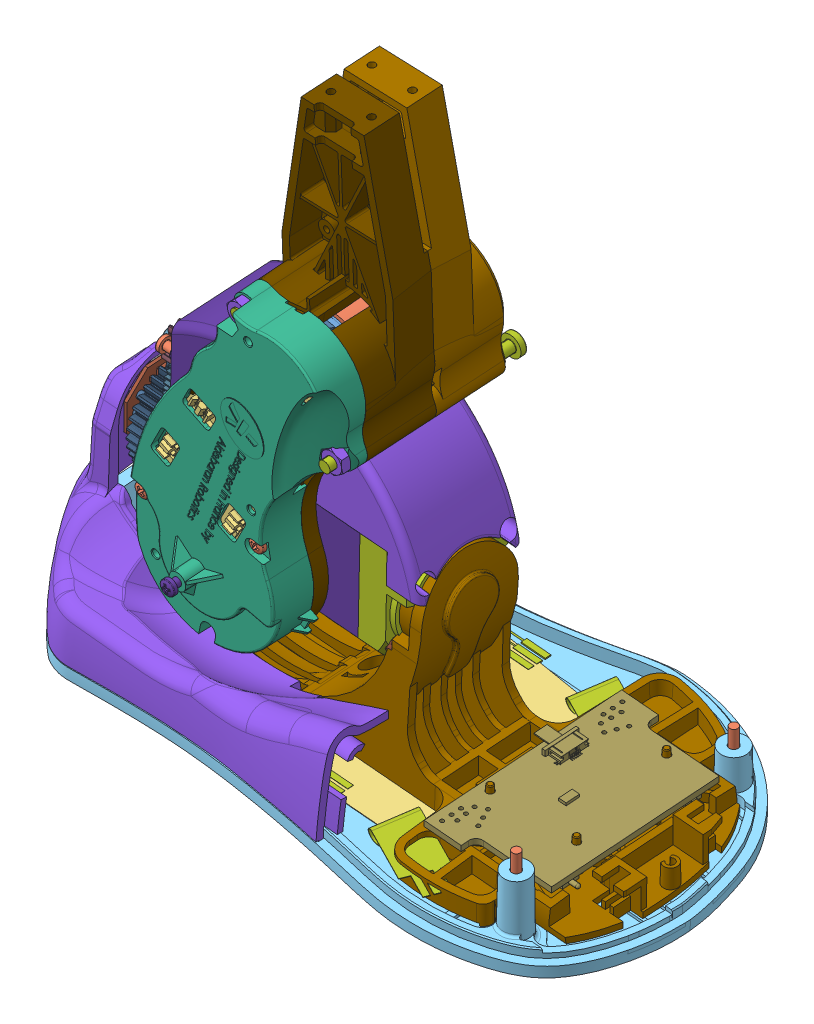
SolidWorks assembly Cheville_Gauche, configuration Défaut. Lengths in mm.
Overall size (176.95 178.66 110.8).
107 component instances, 54 part files, 21 mates.
Components (placement in the parent):
- Pied_Gauche-1: Pied_Gauche [Défaut] at (-33.6626 96.6362 176.8878) size (176.95 81.97 110.8)
  - Left_Foot_jambe droite-1: Left_Foot_jambe droite [Défaut] at (4.3479 -90.4053 5.2353) x (-0.007082 -0.079671 0.996796) z (-0.996073 0.088539 0) size (106.44 58.7 171.69)
    - STD_M850001__P_Scotch_double_Face_3M_5419_Default-1: STD_M850001__P_Scotch_double_Face_3M_5419_Default [Default] at (-23.9002 -40.8442 -61.9998) x (0 0 -1) z (0 1 0) size (13 10 0.25)
    - STD_M700004__PZ99_KA22x8_KA22 x 8-1: STD_M700004__PZ99_KA22x8_KA22 x 8 [Default] at (-16.4 -30.0842 45.1) x (0 1 0) z (-0.943584 0 -0.331134) size (9.5 3.9 3.91)
    - STD_M850001__P_Scotch_double_Face_3M_5419_Default-2: STD_M850001__P_Scotch_double_Face_3M_5419_Default [Default] at (27.1002 -40.5942 -74.9998) x (0 0 1) z (0 -1 0) size (13 10 0.25)
    - STD_E990013__P_FSR_4P-1: STD_E990013__P_FSR_4P [Default] at (19.0956 -40.8442 30.9044) x (0 0 1) z (0 -1 0) size (108.1 14 0.37)
    - STD_M700004__PZ99_KA22x8_KA22 x 8-2: STD_M700004__PZ99_KA22x8_KA22 x 8 [Default] at (13.2 -30.0842 45.1) x (0 1 0) z (-0.676128 0 -0.736784) size (9.5 3.9 3.91)
    - STD_M830010__P_Axial_Magnet_6x3_Default-1: STD_M830010__P_Axial_Magnet_6x3_Default [Default] at (-0.0436 -43.3342 -16.4801) x (0.495785 0 -0.868445) z (0 1 0) size (6 6 3.01)
    - ALD_M010097__P_semelle_gauche_default-1: ALD_M010097__P_semelle_gauche_default [Default] at (0 -45.0842 21.6) x (0 0 -1) z (0 1 0) size (171.69 106.44 28.07)
    - STD_M850001__P_Scotch_double_Face_3M_5419_Default-3: STD_M850001__P_Scotch_double_Face_3M_5419_Default [Default] at (-24.4459 -40.8442 37.9999) x (0.087156 0 -0.996195) z (0 1 0) size (13 10 0.25)
    - STD_M510003__P_palier_GFM_1012-07_stabdard-1: STD_M510003__P_palier_GFM_1012-07_stabdard [Default] at (0 0 31.4) x (0 0 1) z (-0.219796 0.975546 0) size (7 18 18)
    - STD_M850001__P_Scotch_double_Face_3M_5419_Default-4: STD_M850001__P_Scotch_double_Face_3M_5419_Default [Default] at (13.1002 -40.8442 36.8998) x (1 0 0) z (0 1 0) size (13 10 0.25)
    - STD_E990012__P_FSR_2P_pli 4-1: STD_E990012__P_FSR_2P_pli 4 [Default] at (23.0956 -40.8442 -69.0044) x (0 0 -1) z (0 -1 0) size (57.3 20.1 4.54)
    - ALD_M010133__P_coque_interieure_pied_gauche-1: ALD_M010133__P_coque_interieure_pied_gauche [Default] at (0 -45.0842 21.6) x (0 0 -1) z (0 1 0) size (104.04 41.95 56.84)
    - STD_M700004__PZ99_KA22x8_KA22 x 8-3: STD_M700004__PZ99_KA22x8_KA22 x 8 [Default] at (-4.25 -31.212 18.3352) x (0 0 1) z (0.021347 -0.999772 0) size (9.5 3.9 3.91)
    - ALD_M010099__P_structure_pied_gauche_default-1: ALD_M010099__P_structure_pied_gauche_default [Default] at (-6.6116 -41.5942 -17.9596) x (0 1 0) z (0 0 -1) size (54.34 78.21 137.68)
    - STD_M700004__PZ99_KA22x8_KA22 x 8-4: STD_M700004__PZ99_KA22x8_KA22 x 8 [Default] at (4.25 -31.212 18.3521) x (0 0 1) z (0.183952 -0.982935 0) size (9.5 3.9 3.91)
    - ALD_M010018__P_support_dente_A08-1: ALD_M010018__P_support_dente_A08 [Default] at (0 0 31.2) x (0 0 -1) z (-1 0 0) size (20.4 48.62 27.24)
    - STD_M700004__PZ99_KA22x8_KA22 x 8-5: STD_M700004__PZ99_KA22x8_KA22 x 8 [Default] at (26.7 -30.0842 -81.8) x (0 1 0) z (-0.96573 0 -0.25955) size (9.5 3.9 3.91)
    - STD_M700004__PZ99_KA22x8_KA22 x 8-6: STD_M700004__PZ99_KA22x8_KA22 x 8 [Default] at (-31.7 -35.0842 -81.8) x (0 1 0) z (-0.841418 0 -0.540385) size (9.5 3.9 3.91)
    - STD_M830010__P_Axial_Magnet_6x3_Default-2: STD_M830010__P_Axial_Magnet_6x3_Default [Default] at (-0.0436 -39.0942 -16.4801) x (-0.919248 0 0.393679) z (0 1 0) size (6 6 3.01)
    - STD_E990013__P_FSR_4P-2: STD_E990013__P_FSR_4P [Default] at (-29.896 -40.8442 31.5047) x (-0.087156 0 0.996195) z (0 -1 0) size (108.1 14 0.37)
    - ALD_E000030__P_carte_MRE-1: ALD_E000030__P_carte_MRE [Default] at (10 10 41.9) x (0 -1 0) z (0 0 -1) size (18.94 18.94 5)
    - STD_E990012__P_FSR_2P_pli 4-2: STD_E990012__P_FSR_2P_pli 4 [Default] at (-29.8956 -40.8442 -69.0068) x (0 0 -1) z (0 -1 0) size (57.3 20.1 4.54)
    - ALD_E000032__P_Carte_Moteur_Pied_A00-1: ALD_E000032__P_Carte_Moteur_Pied_A00 [Default] at (19.9576 -32.4942 -54.2074) size (53 5.6 34.31)
- Articulation-1: Articulation [Défaut] at (-33.1516 96.7388 183.0978) x (0.999981 -0.000211 0.00612) z (-0.00612 -0.068846 0.997609) size (89.94 67.22 56.71)
  - STD_M510004__P_palier_GFM_1517-05_stabdard-1: STD_M510004__P_palier_GFM_1517-05_stabdard [Default] at (2.8538 -90.2725 -9.0647) x (0 0 -1) z (0.822457 -0.568828 0) size (5 23 23)
  - STD_M510004__P_palier_GFM_1517-05_stabdard-2: STD_M510004__P_palier_GFM_1517-05_stabdard [Default] at (2.8538 -90.2725 19.5353) x (0 0 1) z (-0.611916 -0.790923 0) size (5 23 23)
  - STD_M700004__PZ99_KA22x8_KA22 x 8-1: STD_M700004__PZ99_KA22x8_KA22 x 8 [Default] at (-24.1951 -60.2597 16.5853) x (0.996073 -0.088539 0) z (-0.057058 -0.641904 0.764659) size (9.5 3.9 3.91)
  - ALD_M100016__P_axe_3x27_3-1: ALD_M100016__P_axe_3x27_3 [Default] at (-34.4823 -70.3887 5.2353) x (0.020016 0.225177 0.974112) z (0.996073 -0.088539 0) size (3 3 27.3)
  - STD_M700004__PZ99_KA22x8_KA22 x 8-2: STD_M700004__PZ99_KA22x8_KA22 x 8 [Default] at (-27.3825 -96.1183 16.5853) x (0.996073 -0.088539 0) z (0.083377 0.937999 0.336461) size (9.5 3.9 3.91)
  - STD_M700004__PZ99_KA22x8_KA22 x 8-3: STD_M700004__PZ99_KA22x8_KA22 x 8 [Default] at (-27.6481 -99.1066 5.2353) x (0.996073 -0.088539 0) z (-0.010813 -0.12165 0.992514) size (9.5 3.9 3.91)
  - STD_M700004__PZ99_KA22x8_KA22 x 8-4: STD_M700004__PZ99_KA22x8_KA22 x 8 [Default] at (-27.3825 -96.1183 -6.1147) x (0.996073 -0.088539 0) z (0.082869 0.932287 0.352099) size (9.5 3.9 3.91)
  - ALD_M010033__P_couvercle_X_AV_cheville_A02-1: ALD_M010033__P_couvercle_X_AV_cheville_A02 [Default] at (-8.5612 -86.5472 -8.8647) x (-0.996073 0.088539 0) z (0 0 -1) size (18.62 54.33 28.93) (hidden)
  - STD_M700002__P_KA22x14-1: STD_M700002__P_KA22x14 [Default] at (42.8327 -82.1189 16.3353) x (-0.996073 0.088539 0) z (0 0 -1) size (15.5 3.9 3.91)
  - ALD_M100015__P_axe_2x13-1: ALD_M100015__P_axe_2x13 [Default] at (-27.6393 -85.4537 5.2353) x (-0.085413 -0.960907 -0.263366) z (0.996073 -0.088539 0) size (2 2 13)
  - ALD_M010030__P_cage_fut_moteur_cheville_gauche_Axx-1: ALD_M010030__P_cage_fut_moteur_cheville_gauche_Axx [Default] at (72.1207 -93.7188 5.2353) x (0 0 1) z (-0.996073 0.088539 0) size (43 61.38 54.3)
  - ALD_M100004__P_axe_Y_B00-1: ALD_M100004__P_axe_Y_B00 [Default] at (2.8538 -90.2725 -10.1647) x (-0.056962 -0.998376 0) z (0.998376 -0.056962 0) size (4 18.6 4)
  - STD_M710004__P_vis_M2x5_ALD_M710004__PZ99_vis_M2x5-1: STD_M710004__P_vis_M2x5_ALD_M710004__PZ99_vis_M2x5 [Default] at (-11.7545 -89.7184 10.1502) x (0.996073 -0.088539 0) z (0.051152 0.575461 -0.816228) size (6.41 3.8 3.8)
  - ALD_E000030__P_carte_MRE-1: ALD_E000030__P_carte_MRE [Default] at (34.1593 -80.3051 15.2353) x (0 0 -1) z (-0.996073 0.088539 0) size (18.94 18.94 5)
  - ALD_M010292__P_Motor_Ring_Default-1: ALD_M010292__P_Motor_Ring_Default [Default] at (20.5241 -89.1325 5.2353) x (0.032389 0.364381 0.930686) z (-0.996073 0.088539 0) size (24 24 29.5)
  - ALD_M080003__P_rondelle_flex_X_cheville_A00-1: ALD_M080003__P_rondelle_flex_X_cheville_A00 [Default] at (44.0414 -93.9336 5.2353) x (0 0 1) z (-0.996073 0.088539 0) size (16 16 0.25)
  - STD_M710004__P_vis_M2x5_ALD_M710004__PZ99_vis_M2x5-2: STD_M710004__P_vis_M2x5_ALD_M710004__PZ99_vis_M2x5 [Default] at (-11.1451 -82.8625 0.3204) x (0.996073 -0.088539 0) z (0.012858 0.144656 -0.989398) size (6.41 3.8 3.8)
  - ALD_M840030__P_Portescap_22NT_82_213P_Z13_Default-1: ALD_M840030__P_Portescap_22NT_82_213P_Z13_Default [Default] at (21.0222 -89.1768 5.2353) x (-0.037418 -0.420959 -0.906308) z (0.080244 0.902748 -0.422618) size (22 50.65 22)
  - STD_M710004__P_vis_M2x5_ALD_M710004__PZ99_vis_M2x5-3: STD_M710004__P_vis_M2x5_ALD_M710004__PZ99_vis_M2x5 [Default] at (-11.2253 -83.7647 10.6731) x (0.996073 -0.088539 0) z (-0.004205 -0.047303 0.998872) size (6.41 3.8 3.8)
  - ALD_M010053__P_support_aimant-1: ALD_M010053__P_support_aimant [Default] at (23.4127 -89.3893 5.2353) x (0.029754 0.33473 -0.941844) z (-0.08339 -0.938145 -0.33605) size (7.64 6.4 7.6)
  - STD_M700004__PZ99_KA22x8_KA22 x 8-5: STD_M700004__PZ99_KA22x8_KA22 x 8 [Default] at (36.5653 -101.8026 16.5853) x (-0.996073 0.088539 0) z (-0.071881 -0.808671 0.583852) size (9.5 3.9 3.91)
  - ALD_M010053__P_support_aimant-2: ALD_M010053__P_support_aimant [Default] at (-28.5225 -87.4835 5.2353) x (-0.076677 -0.862624 -0.5) z (0.04427 0.498036 -0.866025) size (7.64 6.4 7.6)
  - STD_M700004__PZ99_KA22x8_KA22 x 8-6: STD_M700004__PZ99_KA22x8_KA22 x 8 [Default] at (36.5653 -101.8026 -6.1147) x (-0.996073 0.088539 0) z (0.015883 0.17868 0.983779) size (9.5 3.9 3.91)
  - ALD_M010201__P_magnet_wires_support-1: ALD_M010201__P_magnet_wires_support [Default] at (2.8538 -90.2725 21.5353) x (0.996073 -0.088539 0) z (-0.088539 -0.996073 0) size (14 6.41 14)
  - STD_M700002__P_KA22x14-2: STD_M700002__P_KA22x14 [Default] at (42.8327 -82.1189 -5.8647) x (-0.996073 0.088539 0) z (0.008404 0.094544 0.995485) size (15.5 3.9 3.91)
  - STD_M700004__PZ99_KA22x8_KA22 x 8-7: STD_M700004__PZ99_KA22x8_KA22 x 8 [Default] at (36.2997 -104.7908 5.2353) x (-0.996073 0.088539 0) z (-0.032778 -0.368759 0.928947) size (9.5 3.9 3.91)
  - ALD_M010035__P_couvercle_X_AR_Axx-1: ALD_M010035__P_couvercle_X_AR_Axx [Default] at (29.5884 -89.9382 5.2353) x (0 0 -1) z (0.996073 -0.088539 0) size (28.83 33.93 15.89)
  - STD_M700004__PZ99_KA22x8_KA22 x 8-8: STD_M700004__PZ99_KA22x8_KA22 x 8 [Default] at (-24.1951 -60.2597 -6.1147) x (0.996073 -0.088539 0) z (-0.056918 -0.640333 0.765986) size (9.5 3.9 3.91)
  - ALD_M010055__P_cache_fut_moteur_cheville_A-1: ALD_M010055__P_cache_fut_moteur_cheville_A [Default] at (72.1207 -93.7188 19.3353) x (0.996073 -0.088539 0) z (0 0 1) size (45.42 37.32 28.46)
  - ALD_M010016__P_roue_sortie_inf-1: ALD_M010016__P_roue_sortie_inf [Default] at (2.8538 -90.2725 -14.0647) x (0.994803 -0.101815 0) z (0.101815 0.994803 0) size (27.24 12.9 27.24)
- Moteur_R-1: Moteur_R [Default] at (-11.9438 7.391 182.3097) x (-0.015052 -0.169331 -0.985444) z (0.08725 0.981574 -0.169999) size (4.5 3.4 4.5)
- Pignon1_R-1: Pignon1_R [Default] at (-43.6949 24.0346 183.2635) x (0.085449 0.961307 -0.261892) z (0.023188 0.260863 0.965097) size (24.51 6.7 24.51)
- Pignon2_R-1: Pignon2_R [Default] at (-49.9472 10.1682 182.2682) x (-0.079826 -0.898046 -0.432598) z (0.038302 0.430899 -0.901587) size (19.63 8.2 19.62)
- Pignon3_R-1: Pignon3_R [Défaut] at (-29.355 99.163 176.5268) size (16.48 30.2 29.81)
  - ALD_M100067__P_Pinion_Inf_3_A00-1: ALD_M100067__P_Pinion_Inf_3_A00 [Default] at (-23.5038 -74.3138 6.7368) x (-0.087964 -0.989599 -0.113825) z (0.010078 0.113377 -0.993501) size (8.58 13 8.96)
  - ALD_M010288__P_Inf_Wheel_3&4_A00-1: ALD_M010288__P_Inf_Wheel_3&4_A00 [Default] at (-21.8104 -74.4643 6.7368) x (-0.021769 -0.244907 -0.969302) z (0.085821 0.965495 -0.245872) size (24.52 5.6 24.55)
  - ALD_M010289__P_Inf_Limiter_Default-1: ALD_M010289__P_Inf_Limiter_Default [Default] at (-23.4042 -74.3227 6.7368) x (-0.010078 -0.113377 0.993501) z (-0.996073 0.088539 0) size (16.14 19.2 3.9)
- Tibia_Seul-1: Tibia_Seul [Défaut] at (-11.3364 94.7571 183.2953) x (0.970622 -0.240376 -0.010635) z (-0.00612 -0.068846 0.997609) size (51.2 135.49 82.15)
  - STD_M700013__PZ99_KA22x5_KA22 x 6-1: STD_M700013__PZ99_KA22x5_KA22 x 6 [Default] at (16.9636 -10.9615 1.7353) x (0 0 1) z (0.337513 -0.941321 0) size (6.5 3.9 3.91)
  - STD_M700003__PZ99_KA22x6_KA22 x 6-1: STD_M700003__PZ99_KA22x6_KA22 x 6 [Default] at (2.1457 -91.3172 43.0853) x (0 0 -1) z (0.448628 -0.893719 0) size (7.5 3.9 3.91)
  - ALD_M010048__P_couvercle_tibia_meca_gauche_Axx-1: ALD_M010048__P_couvercle_tibia_meca_gauche_Axx [Default] at (2.8538 9.7275 -12.4647) x (0 -1 0) z (0 0 1) size (91.48 47.32 23.1) (hidden)
  - ALD_M010046__P_boitier_tibia_elec_gauche_ALD_M010046__PAxx_boitier_elec_gauche-1: ALD_M010046__P_boitier_tibia_elec_gauche_ALD_M010046__PAxx_boitier_elec_gauche [Default] at (2.8538 9.7275 5.2353) x (0 -1 0) z (0 0 1) size (135.22 47.39 29.9)
  - STD_M700013__PZ99_KA22x5_KA22 x 6-2: STD_M700013__PZ99_KA22x5_KA22 x 6 [Default] at (-1.6212 -14.9118 1.7353) x (0 0 1) z (-0.935228 -0.354047 0) size (6.5 3.9 3.91)
  - STD_M710004__P_vis_M2x5_ALD_M710004__PZ99_vis_M2x5-1: STD_M710004__P_vis_M2x5_ALD_M710004__PZ99_vis_M2x5 [Default] at (10.4845 -27.6822 -14.6647) x (0 0 1) z (0.702902 0.711287 0) size (6.41 3.8 3.8)
  - ALD_M840031-1: ALD_M840031 [Default] at (12.0374 -33.4777 18.7353) x (-0.707107 -0.707107 0) z (0.707107 -0.707107 0) size (22 50.65 22)
  - STD_M700005__PZ99_KA22x12_Default-1: STD_M700005__PZ99_KA22x12_Default [Default] at (14.3538 -74.4725 34.0353) x (0 0 -1) z (0.975434 -0.220294 0) size (13.5 3.9 3.91)
  - STD_M710004__P_vis_M2x5_ALD_M710004__PZ99_vis_M2x5-2: STD_M710004__P_vis_M2x5_ALD_M710004__PZ99_vis_M2x5 [Default] at (17.8329 -35.0307 -14.6647) x (0 0 1) z (0.331606 0.943418 0) size (6.41 3.8 3.8)
  - ALD_E000183__P_Left_Tibia_Card_Default-1: ALD_E000183__P_Left_Tibia_Card_Default [Default] at (-4.5707 -75.2219 31.3353) x (-0.250739 -0.968055 0) z (0 0 1) size (56.57 25 8.51)
  - STD_M700006__PZ99_KA18x6_Default-1: STD_M700006__PZ99_KA18x6_Default [Default] at (-0.8831 -76.2311 -39.0647) x (0 0 1) z (0.79364 0.608388 0) size (7.2 3.2 3.2)
  - STD_M510004__P_palier_GFM_1517-05_stabdard-1: STD_M510004__P_palier_GFM_1517-05_stabdard [Default] at (2.8538 -90.2725 -9.0647) x (0 0 -1) z (0.822457 -0.568828 0) size (5 23 23)
  - STD_M510004__P_palier_GFM_1517-05_stabdard-2: STD_M510004__P_palier_GFM_1517-05_stabdard [Default] at (2.8538 -90.2725 19.5353) x (0 0 1) z (-0.611916 -0.790923 0) size (5 23 23)
  - ALD_E000030__P_carte_MRE-1: ALD_E000030__P_carte_MRE [Default] at (-7.1462 -100.2725 30.9353) x (0 1 0) z (0 0 -1) size (18.94 18.94 5)
  - ALD_M100018__P_axe_3x20_2-1: ALD_M100018__P_axe_3x20_2 [Default] at (-2.245 -74.58 -29.5647) x (-0.898721 -0.43852 0) z (0 0 1) size (3 3 20)
  - ALD_M010050__P_couvercle_tibia_elec_gauche_Axx-1: ALD_M010050__P_couvercle_tibia_elec_gauche_Axx [Default] at (3.2067 9.6772 24.5353) x (-0.010505 -0.999945 0) z (0 0 1) size (91.58 50.24 17.3)
  - STD_M700005__PZ99_KA22x12_Default-2: STD_M700005__PZ99_KA22x12_Default [Default] at (-15.1462 -84.8725 -22.6647) x (0 0 1) z (-0.865979 -0.500081 0) size (13.5 3.9 3.91)
  - STD_M710005__PZ99_Vis_M3x50_ISO 7045 - M3 x 50-1: STD_M710005__PZ99_Vis_M3x50_ISO 7045 - M3 x 50 [Default] at (-1.7576 -23.8893 -20.5647) x (0 0 1) z (0.06312 0.998006 0) size (52.4 5.6 5.68)
  - STD_M700005__PZ99_KA22x12_Default-3: STD_M700005__PZ99_KA22x12_Default [Default] at (-15.1462 -84.8725 34.0353) x (0 0 -1) z (-0.568693 -0.82255 0) size (13.5 3.9 3.91)
  - STD_M710002__P_ecrou_M3-1: STD_M710002__P_ecrou_M3 [Default] at (25.8324 -43.0662 29.9353) x (0.734221 -0.678911 0) z (0 0 1) size (5.5 6.35 2.4)
  - STD_M700005__PZ99_KA22x12_Default-4: STD_M700005__PZ99_KA22x12_Default [Default] at (-12.1462 -61.8725 -22.6647) x (0 0 1) z (-0.987069 0.160297 0) size (13.5 3.9 3.91)
  - STD_M710005__PZ99_Vis_M3x50_ISO 7045 - M3 x 50-2: STD_M710005__PZ99_Vis_M3x50_ISO 7045 - M3 x 50 [Default] at (25.8324 -43.0662 -20.5647) x (0 0 1) z (-0.935181 -0.354169 0) size (52.4 5.6 5.68)
  - STD_M700005__PZ99_KA22x12_Default-5: STD_M700005__PZ99_KA22x12_Default [Default] at (5.8538 -107.2725 -22.6647) x (0 0 1) z (0.139397 0.990237 0) size (13.5 3.9 3.91)
  - ALD_M010292__P_Motor_Ring_Default-1: ALD_M010292__P_Motor_Ring_Default [Default] at (12.0374 -33.4777 -11.2647) x (0.565934 0.824451 0) z (0 0 1) size (24 24 29.5)
  - ALD_M010044__P_boitier_tibia_meca_gauche_ALD_M010044__PAxx_boitier_tibia_meca_gauche-1: ALD_M010044__P_boitier_tibia_meca_gauche_ALD_M010044__PAxx_boitier_tibia_meca_gauche [Default] at (2.8538 9.7275 5.2353) x (0 -1 0) z (0 0 1) size (135.22 47.39 25.5)
  - STD_M510002__P_palier_GSM_0405-04-1: STD_M510002__P_palier_GSM_0405-04 [Default] at (2.8538 -90.2725 -28.7647) x (0.409552 -0.912287 0) z (0 0 1) size (5.5 5.5 4)
  - ALD_M100021__P_axe_3x11_7-1: ALD_M100021__P_axe_3x11_7 [Default] at (6.6023 -47.3511 -22.7647) x (-0.979613 0.200892 0) z (0 0 1) size (3 3 11.7)
  - ALD_M010053__P_support_aimant-1: ALD_M010053__P_support_aimant [Default] at (12.0374 -33.4777 20.4853) x (0.99932 -0.036877 0) z (-0.036877 -0.99932 0) size (7.64 6.4 7.6)
  - STD_M710004__P_vis_M2x5_ALD_M710004__PZ99_vis_M2x5-3: STD_M710004__P_vis_M2x5_ALD_M710004__PZ99_vis_M2x5 [Default] at (6.2418 -31.9248 -14.6647) x (0 0 1) z (-0.85095 0.525247 0) size (6.41 3.8 3.8)
  - ALD_M100017__P_axe_2x19_7-1: ALD_M100017__P_axe_2x19_7 [Default] at (1.2276 -60.6565 -29.2647) x (-0.661597 -0.749859 0) z (0 0 1) size (2 2 19.7)
  - STD_M710002__P_ecrou_M3-2: STD_M710002__P_ecrou_M3 [Default] at (-1.7576 -23.8893 31.4353) x (-0.847827 0.530273 0) z (0 0 1) size (5.5 6.35 2.4)
  - STD_M700004__PZ99_KA22x8_KA22 x 8-2: STD_M700004__PZ99_KA22x8_KA22 x 8 [Default] at (5.8538 -107.2725 30.5353) x (0 0 -1) z (0.402889 -0.915249 0) size (9.5 3.9 3.91)
  - STD_M700005__PZ99_KA22x12_Default-6: STD_M700005__PZ99_KA22x12_Default [Default] at (14.3538 -74.4725 -22.6647) x (0 0 1) z (0.865979 0.500081 0) size (13.5 3.9 3.91)
- Pignon1_T-1: Pignon1_T [Défaut] at (-4.033 93.4122 183.2473) x (0.921662 -0.387421 -0.021083) z (-0.00612 -0.068846 0.997609) size (34 34 6.7)
  - ALD_M010013__P_mobile_inf_1_A00-1: ALD_M010013__P_mobile_inf_1_A00 [Default] at (6.6023 -47.3511 -13.8647) x (-0.555489 0.831524 0) z (-0.831524 -0.555489 0) size (24.51 6.7 24.51)
- Moteur_T-1: Moteur_T [Défaut] at (-19.7494 92.8501 183.1121) x (0.999981 -0.000211 0.00612) z (-0.00612 -0.068846 0.997609) size (7.73 7.74 3.4)
  - ALD6667-1: ALD6667 [Default] at (12.0374 -33.4777 -12.6647) x (-0.191867 -0.981421 0) z (0.981421 -0.191867 0) size (6.6 3.4 6.59)
- Pignon2_T-1: Pignon2_T [Défaut] at (-50.4252 90.5736 182.7668) x (0.914281 0.403696 0.033468) z (-0.00612 -0.068846 0.997609) size (26.24 26.25 8.2)
  - ALD_M010014__P_mobile_inf_2_A00-1: ALD_M010014__P_mobile_inf_2_A00 [Default] at (1.2276 -60.6565 -18.3647) x (0.438964 -0.898505 0) z (0.898505 0.438964 0) size (19.63 8.2 19.62)
- Pignon3_T-1: Pignon3_T [Défaut] at (-15.6945 95.8364 183.343) x (0.983332 -0.181702 -0.006507) z (-0.00612 -0.068846 0.997609) size (31.84 31.83 12.1)
  - ALD_M100068__P_Pinion_inf_4_A00-1: ALD_M100068__P_Pinion_inf_4_A00 [Default] at (-2.245 -74.58 -24.3647) x (0.042959 -0.999077 0) z (-0.999077 -0.042959 0) size (8.58 10.5 8.96)
  - ALD_M010289__P_Inf_Limiter_Default-1: ALD_M010289__P_Inf_Limiter_Default [Default] at (-2.245 -74.58 -24.4647) x (0.999077 0.042959 0) z (0 0 1) size (16.14 19.2 3.9)
  - ALD_M010288__P_Inf_Wheel_3&4_A00-1: ALD_M010288__P_Inf_Wheel_3&4_A00 [Default] at (-2.245 -74.58 -25.8647) x (0.367326 -0.930092 0) z (-0.930092 -0.367326 0) size (24.52 5.6 24.55)
Mates (geometry in assembly coordinates):
- Coaxiale1: concentric aligned: cylinder of Pied_Gauche-1/Left_Foot_jambe droite-1/STD_M510003__P_palier_GFM_1012-07_stabdard-1 through (935.4813 -79.528 182.1231) axis (0.996073 -0.088539 0) radius 5; cylinder of Articulation-1/ALD_M010033__P_couvercle_X_AV_cheville_A02-1 through (-67.5639 9.6308 182.1231) axis (0.996073 -0.088539 0) radius 5
- Coïncidente1: coincident anti-aligned: plane of Pied_Gauche-1/Left_Foot_jambe droite-1/STD_M510003__P_palier_GFM_1012-07_stabdard-1 through (-60.479 10.2756 191.0331) normal (0.996073 -0.088539 0); plane of Articulation-1/ALD_M010033__P_couvercle_X_AV_cheville_A02-1 through (-60.5914 9.0111 182.1231) normal (-0.996073 0.088539 0)
- Coaxiale2: concentric aligned: cylinder of Articulation-1/ALD_M840030__P_Portescap_22NT_82_213P_Z13_Default-1 through (-47.404 10.543 182.3097) axis (0.996073 -0.088539 0) radius 1; cylinder of Moteur_R-1 through (-46.8063 10.4899 182.3097) axis (0.996073 -0.088539 0) radius 1
- Coïncidente2: coincident anti-aligned: plane of Articulation-1/ALD_M840030__P_Portescap_22NT_82_213P_Z13_Default-1 through (-43.4197 10.1889 182.3097) normal (-0.996073 0.088539 0); plane of Moteur_R-1 through (-43.4197 10.1889 182.3097) normal (0.996073 -0.088539 0)
- Coaxiale3: concentric anti-aligned: cylinder of Articulation-1/ALD_M100016__P_axe_3x27_3-1 through (-40.4576 23.7469 183.2635) axis (-0.996073 0.088539 0) radius 1.5; cylinder of Pignon1_R-1 through (-43.6949 24.0346 183.2635) axis (0.996073 -0.088539 0) radius 1.5
- Coaxiale4: concentric anti-aligned: cylinder of Articulation-1/ALD_M100015__P_axe_2x13-1 through (-47.8554 9.9822 182.2682) axis (-0.996073 0.088539 0) radius 1; cylinder of Pignon2_R-1 through (-49.9472 10.1682 182.2682) axis (0.996073 -0.088539 0) radius 1
- Distance1: distance = 6 mm anti-aligned: plane of Articulation-1/ALD_M010033__P_couvercle_X_AV_cheville_A02-1 through (-58.1012 8.7897 182.1231) normal (0.996073 -0.088539 0); plane of Pignon2_R-1 through (-52.611 2.7882 178.6279) normal (-0.996073 0.088539 0)
- Coïncidente4: coincident anti-aligned: cylinder of Articulation-1/ALD_M100016__P_axe_3x27_3-1 through (-40.4576 23.7469 183.2635) axis (-0.996073 0.088539 0) radius 1.5; circle of Pignon3_R-1/ALD_M100067__P_Pinion_Inf_3_A00-1
- Coaxiale5: concentric anti-aligned: cylinder of Articulation-1/ALD_M100016__P_axe_3x27_3-1 through (-40.4576 23.7469 183.2635) axis (-0.996073 0.088539 0) radius 1.5; cylinder of Pignon3_R-1/ALD_M100067__P_Pinion_Inf_3_A00-1 through (-52.8588 24.8492 183.2635) axis (0.996073 -0.088539 0) radius 1.5
- Coïncidente5: coincident anti-aligned: plane of Articulation-1/ALD_M010033__P_couvercle_X_AV_cheville_A02-1 through (-58.1012 8.7897 182.1231) normal (0.996073 -0.088539 0); plane of Pignon3_R-1/ALD_M010288__P_Inf_Wheel_3&4_A00-1 through (-56.8819 22.5076 172.6642) normal (-0.996073 0.088539 0)
- Distance2: distance = 11 mm anti-aligned: plane of Pignon1_R-1 through (-44.7364 34.9062 180.35) normal (-0.996073 0.088539 0); plane of Articulation-1/ALD_M010033__P_couvercle_X_AV_cheville_A02-1 through (-58.1012 8.7897 182.1231) normal (0.996073 -0.088539 0)
- Coaxiale6: concentric aligned: cylinder of Articulation-1/ALD_M100004__P_axe_Y_B00-1 through (-36.3362 -61.4663 1164.3684) axis (-0.00612 -0.068846 0.997609) radius 2; cylinder of Tibia_Seul-1/STD_M510004__P_palier_GFM_1517-05_stabdard-1 through (-36.3441 -61.5558 1165.6653) axis (-0.00612 -0.068846 0.997609) radius 7.5
- Distance3: distance = 0.6 mm anti-aligned: plane of Articulation-1/ALD_M010030__P_cage_fut_moteur_cheville_gauche_Axx-1 through (-51.8738 34.8002 198.0901) normal (-0.00612 -0.068846 0.997609); plane of Tibia_Seul-1/ALD_M010046__P_boitier_tibia_elec_gauche_ALD_M010046__PAxx_boitier_elec_gauche-1 through (-98.7132 47.4851 199.2796) normal (0.00612 0.068846 -0.997609)
- Coaxiale7: concentric aligned: cylinder of Tibia_Seul-1/ALD_M840031-1 through (-7.6032 60.5966 164.2561) axis (-0.00612 -0.068846 0.997609) radius 1; cylinder of Moteur_T-1/ALD6667-1 through (-7.6277 60.3212 168.2465) axis (-0.00612 -0.068846 0.997609) radius 1
- Coïncidente9: coincident anti-aligned: plane of Tibia_Seul-1/ALD_M840031-1 through (-7.6277 60.3212 168.2465) normal (0.00612 0.068846 -0.997609); plane of Moteur_T-1/ALD6667-1 through (-7.8194 59.3422 168.1778) normal (-0.00612 -0.068846 0.997609)
- Coaxiale8: concentric anti-aligned: cylinder of Tibia_Seul-1/ALD_M100021__P_axe_3x11_7-1 through (-16.2499 48.0849 168.953) axis (0.00612 0.068846 -0.997609) radius 1.5; cylinder of Pignon1_T-1/ALD_M010013__P_mobile_inf_1_A00-1 through (-16.2328 48.2776 166.1597) axis (-0.00612 -0.068846 0.997609) radius 1.5
- Coïncidente10: coincident anti-aligned: plane of Tibia_Seul-1/ALD_M010044__P_boitier_tibia_meca_gauche_ALD_M010044__PAxx_boitier_tibia_meca_gauche-1 through (-16.2334 48.2708 166.2595) normal (0.00612 0.068846 -0.997609); plane of Pignon1_T-1/ALD_M010013__P_mobile_inf_1_A00-1 through (-16.2334 48.2708 166.2595) normal (-0.00612 -0.068846 0.997609)
- Coaxiale9: concentric anti-aligned: cylinder of Tibia_Seul-1/ALD_M100017__P_axe_2x19_7-1 through (-24.6763 36.3907 169.5979) axis (0.00612 0.068846 -0.997609) radius 1; cylinder of Pignon2_T-1/ALD_M010014__P_mobile_inf_2_A00-1 through (-24.6224 36.9966 160.8189) axis (-0.00612 -0.068846 0.997609) radius 1
- Coïncidente11: coincident anti-aligned: plane of Tibia_Seul-1/ALD_M010044__P_boitier_tibia_meca_gauche_ALD_M010044__PAxx_boitier_tibia_meca_gauche-1 through (-24.623 36.9897 160.9187) normal (0.00612 0.068846 -0.997609); plane of Pignon2_T-1/ALD_M010014__P_mobile_inf_2_A00-1 through (-24.623 36.9897 160.9187) normal (-0.00612 -0.068846 0.997609)
- Coaxiale10: concentric aligned: cylinder of Tibia_Seul-1/ALD_M100018__P_axe_3x20_2-1 through (-31.3959 23.7442 168.6839) axis (0.00612 0.068846 -0.997609) radius 1.5; cylinder of Pignon3_T-1/ALD_M010288__P_Inf_Wheel_3&4_A00-1 through (-31.2961 24.8664 152.4229) axis (0.00612 0.068846 -0.997609) radius 1.5
- Coïncidente13: coincident anti-aligned: plane of Tibia_Seul-1/ALD_M010044__P_boitier_tibia_meca_gauche_ALD_M010044__PAxx_boitier_tibia_meca_gauche-1 through (-85.1912 37.5463 164.9961) normal (0.00612 0.068846 -0.997609); plane of Pignon3_T-1/ALD_M100068__P_Pinion_inf_4_A00-1 through (-31.3696 24.0403 164.3942) normal (-0.00612 -0.068846 0.997609)
